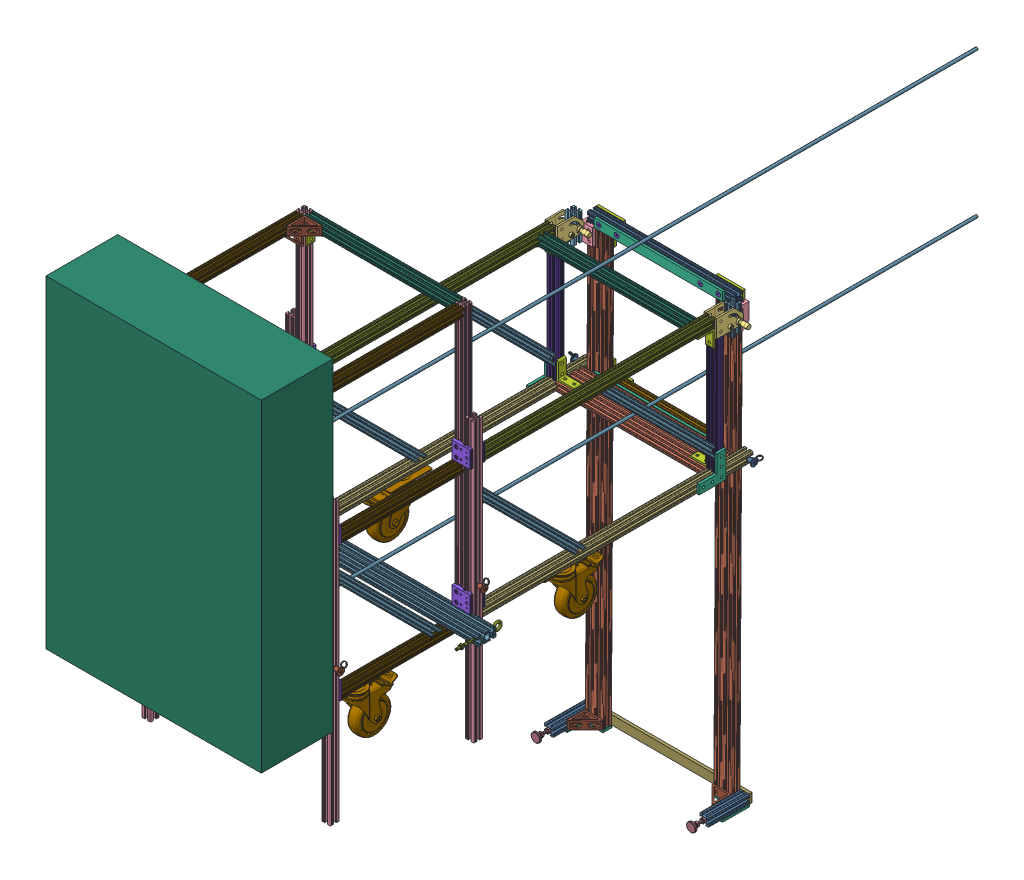
SolidWorks assembly _Tow System Assy V1.1, configuration Default. Lengths in mm.
Overall size (660.4 1762.18 2269.88).
108 component instances, 34 part files, 304 mates.
Components (placement in the parent):
- 8020 -1inch - 0 ft 4.5 in-1: 8020 -1inch - 0 ft 4.5 in [47065T122] at (5.4224 -1222.1152 -947.6338) x (-1 0 0) z (0 0.005452 0.999985) size (25.4 25.4 114.3)
- 8020 -1inch - 0 ft 4.5 in-2: 8020 -1inch - 0 ft 4.5 in [47065T122] at (445.4276 -1222.1152 -947.6338) x (-1 0 0) z (0 0.005452 0.999985) size (25.4 25.4 114.3)
- 47065T125_2inch - 4 ft-1: 47065T125_2inch - 4 ft [47065T125] at (43.5224 -625.4664 -995.3372) x (1 0 0) z (0 0.999985 -0.005452) size (50.8 25.4 1219.2)
- 47065T125_2inch - 4 ft-2: 47065T125_2inch - 4 ft [47065T125] at (407.3276 -625.4664 -995.3372) x (1 0 0) z (0 0.999985 -0.005452) size (50.8 25.4 1219.2)
- 3136N217_Heavy Duty 90 pivot-1: 3136N217_Heavy Duty 90 pivot [3136N217] at (0 -25.4 -927.1) x (-1 0 0) z (0 -1 0) size (70.02 76.2 50.8)
- 47065T953_1in Slider 90 degree-1: 47065T953_1in Slider 90 degree [47065T953] at (41.2872 -39.938 -998.377) x (0 -0.005452 -0.999985) z (0 0.999985 -0.005452) size (41.25 49.99 47.62)
- 47065T953_1in Slider 90 degree-3: 47065T953_1in Slider 90 degree [47065T953] at (409.5628 -39.938 -998.377) x (0 -0.005452 -0.999985) z (0 -0.999985 0.005452) size (41.25 49.99 47.62)
- 3136N217_Heavy Duty 90 pivot-2: 3136N217_Heavy Duty 90 pivot [3136N217] at (450.85 -25.4 -927.1) x (-1 0 0) z (0 -1 0) size (70.02 76.2 50.8)
- 8020 -1inch - 0 ft 3 in-1: 8020 -1inch - 0 ft 3 in [47065T122] at (0 -25.469 -965.1306) x (1 0 0) z (0 -0.999985 0.005452) size (25.4 25.4 76.2)
- 8020 -1inch - 0 ft 3 in-2: 8020 -1inch - 0 ft 3 in [47065T122] at (450.85 -25.469 -965.1306) x (1 0 0) z (0 -0.999985 0.005452) size (25.4 25.4 76.2)
- 1614T644_1in x 364mm Aluminium bar - 5_16 thick-1: 1614T644_1in x 364mm Aluminium bar - 5_16 thick [1614T644] at (225.5224 -380.9144 -980.9702) x (0 -0.999985 0.005452) z (-1 0 0) size (25.4 6 364)
- 1614T644_1in x 364mm Aluminium bar - 5_16 thick-2: 1614T644_1in x 364mm Aluminium bar - 5_16 thick [1614T644] at (225.5224 -3.09 -983.03) x (0 0.999985 -0.005452) z (1 0 0) size (25.4 6 364)
- T Bracket-21: T Bracket [Default] at (119.7224 -381.1039 -1015.7197) x (0 0.999985 -0.005452) z (0 0.005452 0.999985) size (76.2 76.2 6.35)
- T Bracket-22: T Bracket [Default] at (331.1276 -381.1039 -1015.7197) x (0 -0.999985 0.005452) z (0 0.005452 0.999985) size (76.2 76.2 6.35)
- 90585A358_SS Countersunk Screw 1_4-20 x 5-8 in-1: 90585A358_SS Countersunk Screw 1_4-20 x 5-8 in [90585A358] at (56.2224 -380.8981 -977.9703) x (-0.923728 0.383043 -0.002088) z (0 0.005452 0.999985) size (13.49 13.49 16.52)
- 90585A358_SS Countersunk Screw 1_4-20 x 5-8 in-3: 90585A358_SS Countersunk Screw 1_4-20 x 5-8 in [90585A358] at (394.8224 -380.8981 -977.9703) x (-0.923728 0.383043 -0.002088) z (0 0.005452 0.999985) size (13.49 13.49 16.52)
- 90585A358_SS Countersunk Screw 1_4-20 x 5-8 in-4: 90585A358_SS Countersunk Screw 1_4-20 x 5-8 in [90585A358] at (344.0224 -3.0737 -980.0301) x (-0.923728 0.383043 -0.002088) z (0 0.005452 0.999985) size (13.49 13.49 16.52)
- 90585A358_SS Countersunk Screw 1_4-20 x 5-8 in-5: 90585A358_SS Countersunk Screw 1_4-20 x 5-8 in [90585A358] at (344.0224 -380.8981 -977.9703) x (-0.923728 0.383043 -0.002088) z (0 0.005452 0.999985) size (13.49 13.49 16.52)
- 90585A358_SS Countersunk Screw 1_4-20 x 5-8 in-6: 90585A358_SS Countersunk Screw 1_4-20 x 5-8 in [90585A358] at (107.0224 -3.0737 -980.0301) x (-0.923728 0.383043 -0.002088) z (0 0.005452 0.999985) size (13.49 13.49 16.52)
- 90585A358_SS Countersunk Screw 1_4-20 x 5-8 in-7: 90585A358_SS Countersunk Screw 1_4-20 x 5-8 in [90585A358] at (56.2224 -3.0737 -980.0301) x (-0.923728 0.383043 -0.002088) z (0 0.005452 0.999985) size (13.49 13.49 16.52)
- 90585A358_SS Countersunk Screw 1_4-20 x 5-8 in-8: 90585A358_SS Countersunk Screw 1_4-20 x 5-8 in [90585A358] at (107.0224 -380.8981 -977.9703) x (-0.923728 0.383043 -0.002088) z (0 0.005452 0.999985) size (13.49 13.49 16.52)
- 90585A358_SS Countersunk Screw 1_4-20 x 5-8 in-9: 90585A358_SS Countersunk Screw 1_4-20 x 5-8 in [90585A358] at (394.8224 -3.0737 -980.0301) x (-0.923728 0.383043 -0.002088) z (0 0.005452 0.999985) size (13.49 13.49 16.52)
- 8020 -1inch - 1 ft 0.25-3: 8020 -1inch - 1 ft 0.25 [47065T122] at (224.4974 -381 -996.67) x (0 -0.005452 -0.999985) z (1 0 0) size (25.4 25.4 311.15)
- 8020 -1inch - 415mm-1: 8020 -1inch - 415mm [47065T122] at (225.6224 -3.1756 -998.7298) x (0 -0.005452 -0.999985) z (1 0 0) size (25.4 25.4 415)
- 47065T736_ Interior 90 guesset for 1 in-1: 47065T736_ Interior 90 guesset for 1 in [47065T736] at (18.1224 -1220.7008 -979.392) x (0 0.005452 0.999985) z (0 0.999985 -0.005452) size (50.8 50.8 22.23)
- 47065T736_ Interior 90 guesset for 1 in-2: 47065T736_ Interior 90 guesset for 1 in [47065T736] at (432.7276 -1220.7008 -979.392) x (0 0.005452 0.999985) z (0 -0.999985 0.005452) size (50.8 50.8 22.23)
- 1614T644_1in x 465mm Aluminium bar - 5_16 thick-1: 1614T644_1in x 465mm Aluminium bar - 5_16 thick [1614T644] at (225.2224 -1222.4484 -1008.7516) x (0 -0.999985 0.005452) z (-1 0 0) size (25.4 7.94 465)
- 6111K115_SS Leveling Foot-3: 6111K115_SS Leveling Foot [6111K115] at (5.4224 -1221.593 -851.856) x (0.003314 0.99998 -0.005452) z (-0.999995 0.003314 -0.000018) size (25.4 81.68 25.4)
- 6111K115_SS Leveling Foot-4: 6111K115_SS Leveling Foot [6111K115] at (445.4276 -1221.593 -851.856) x (0.316415 0.948607 -0.005172) z (-0.948621 0.316411 -0.001725) size (25.4 81.68 25.4)
- 8020 - 2inch - 2 ft 2 in-1: 8020 - 2inch - 2 ft 2 in [47065T213] at (225.425 -355.6 -165.1) x (0 0 1) z (-1 0 0) size (50.8 25.4 660.4)
- 8020 -1inch - 1 ft 4.75 in-9: 8020 -1inch - 1 ft 4.75 in [47065T122] at (225.425 -381 203.2) x (0 -1 0) z (1 0 0) size (25.4 25.4 425.45)
- 8020 -1inch - 2 ft 3 in-13: 8020 -1inch - 2 ft 3 in [47065T122] at (0 0 -558.8) x (-1 0 0) z (0 0 -1) size (25.4 25.4 685.8)
- 8020 -1inch - 2 ft 3 in-14: 8020 -1inch - 2 ft 3 in [47065T122] at (450.85 0 -558.8) x (-1 0 0) z (0 0 -1) size (25.4 25.4 685.8)
- 8020 -1inch - 1 ft 2 in-1: 8020 -1inch - 1 ft 2 in [47065T122] at (0 -190.5 -914.4) x (1 0 0) z (0 1 0) size (25.4 25.4 355.6)
- 8020 -1inch - 1 ft 3 in-2: 8020 -1inch - 1 ft 3 in [47065T122] at origin size (25.4 25.4 381)
- 8020 -1inch - 1 ft 3 in-3: 8020 -1inch - 1 ft 3 in [47065T122] at (0 -381 0) size (25.4 25.4 381)
- 8020 -1inch - 1 ft 2 in-2: 8020 -1inch - 1 ft 2 in [47065T122] at (450.85 -190.5 -914.4) x (1 0 0) z (0 1 0) size (25.4 25.4 355.6)
- 8020 -1inch - 1 ft 3 in-4: 8020 -1inch - 1 ft 3 in [47065T122] at (450.85 -381 0) size (25.4 25.4 381)
- 8020 -1inch - 1 ft 3 in-6: 8020 -1inch - 1 ft 3 in [47065T122] at (450.85 0 0) size (25.4 25.4 381)
- 8020 -1inch - 1 ft 4.75 in-18: 8020 -1inch - 1 ft 4.75 in [47065T122] at (225.425 0 -863.6) x (0 -1 0) z (1 0 0) size (25.4 25.4 425.45)
- 8020 - 2inch - 1 ft 4.75 in-9: 8020 - 2inch - 1 ft 4.75 in [47065T213] at (225.425 258.3 203.2) x (0 -1 0) z (1 0 0) size (50.8 25.4 425.45)
- 47065T512_8020 - 3inch - 1 ft 4.75 in-1: 47065T512_8020 - 3inch - 1 ft 4.75 in [47065T512] at (225.425 -381 -939.8) x (0 -1 0) z (-1 0 0) size (25.4 76.2 425.45)
- 8020 -1inch - 2 ft 8 inches-1: 8020 -1inch - 2 ft 8 inches [47065T122] at (0 -381 -612.635) size (25.4 25.4 793.47)
- 8020 -1inch - 2 ft 8 inches-2: 8020 -1inch - 2 ft 8 inches [47065T122] at (450.85 -381 -612.635) size (25.4 25.4 793.47)
- 8020 -1inch - 2 ft 7 inches-1: 8020 -1inch - 2 ft 7 inches [47065T122] at (0 0 -203.2) x (-1 0 0) z (0 1 0) size (25.4 25.4 787.4)
- 8020 -1inch - 2 ft 7 inches-2: 8020 -1inch - 2 ft 7 inches [47065T122] at (0 0 203.2) x (-1 0 0) z (0 1 0) size (25.4 25.4 787.4)
- 8020 -1inch - 2 ft 7 inches-3: 8020 -1inch - 2 ft 7 inches [47065T122] at (-29.21 -266.875 -203.3524) x (-1 0 0) z (0 1 0) size (25.4 25.4 787.4)
- 8020 -1inch - 1 ft 3 in-7: 8020 -1inch - 1 ft 3 in [47065T122] at (0 381 0) size (25.4 25.4 381)
- 8020 -1inch - 2 ft 7 inches-6: 8020 -1inch - 2 ft 7 inches [47065T122] at (450.85 0 -203.2) x (-1 0 0) z (0 1 0) size (25.4 25.4 787.4)
- 8020 -1inch - 1 ft 4.75 in-19: 8020 -1inch - 1 ft 4.75 in [47065T122] at (225.425 381 -203.2) x (0 -1 0) z (1 0 0) size (25.4 25.4 425.45)
- 8020 -1inch - 1 ft 4.75 in-20: 8020 -1inch - 1 ft 4.75 in [47065T122] at (225.425 381 203.2) x (0 -1 0) z (1 0 0) size (25.4 25.4 425.45)
- 47065T701_45 Brace - 18 in-12: 47065T701_45 Brace - 18 in [47065T701] at (450.85 -215.6355 -368.5645) x (1 0 0) z (0 0.707107 0.707107) size (25.4 25.56 457.2)
- 8020 -1inch - 2 ft 7 inches-8: 8020 -1inch - 2 ft 7 inches [47065T122] at (450.85 0 203.2) x (-1 0 0) z (0 1 0) size (25.4 25.4 787.4)
- 8020 -1inch - 1 ft 3 in-8: 8020 -1inch - 1 ft 3 in [47065T122] at (450.85 381 0) size (25.4 25.4 381)
- 8020 - 2inch - 1 ft 4.75 in-10: 8020 - 2inch - 1 ft 4.75 in [47065T213] at (225.425 -152.7 203.2) x (0 -1 0) z (1 0 0) size (50.8 25.4 425.45)
- 8020 - 2inch - 1 ft 4.75 in-11: 8020 - 2inch - 1 ft 4.75 in [47065T213] at (225.425 -228.9 203.2) x (0 -1 0) z (1 0 0) size (50.8 25.4 425.45)
- 8020 - 2inch - 1 ft 4.75 in-12: 8020 - 2inch - 1 ft 4.75 in [47065T213] at (225.425 182.1 203.2) x (0 -1 0) z (1 0 0) size (50.8 25.4 425.45)
- L Bracket-13: L Bracket [Default] at (68.9224 -1241.4072 -991.9793) x (0 -0.005452 -0.999985) z (0 0.999985 -0.005452) size (75.8 76.2 6.35)
- L Bracket-15: L Bracket [Default] at (381.9276 -1235.0573 -992.0139) x (0 -0.005452 -0.999985) z (0 -0.999985 0.005452) size (75.8 76.2 6.35)
- T Bracket-17: T Bracket [Default] at (19.05 -317.5 -203.2) x (0 0 -1) z (-1 0 0) size (76.2 76.2 6.35)
- 1 inch x 2 inch L bracket-10: 1 inch x 2 inch L bracket [47065T239] at (12.7 368.3 -204.7875) x (1 0 0) z (0 0 -1) size (50.8 50.8 22.23)
- L Bracket-17: L Bracket [Default] at (-12.7 -317.5 -914.4) x (0 0 -1) z (-1 0 0) size (75.8 76.2 6.35)
- L Bracket-18: L Bracket [Default] at (463.55 -381 -850.9) x (0 -1 0) z (1 0 0) size (75.8 76.2 6.35)
- 1 inch x 2 inch L bracket-39: 1 inch x 2 inch L bracket [47065T239] at (-1.5875 -12.7 -901.7) x (0 0 1) z (1 0 0) size (50.8 50.8 22.23)
- 1 inch x 2 inch L bracket-40: 1 inch x 2 inch L bracket [47065T239] at (452.4375 -12.7 -901.7) x (0 0 1) z (1 0 0) size (50.8 50.8 22.23)
- 1 inch x 2 inch L bracket-44: 1 inch x 2 inch L bracket [47065T239] at (12.7 -368.3 -915.9875) size (50.8 50.8 22.23)
- 1 inch x 2 inch L bracket-45: 1 inch x 2 inch L bracket [47065T239] at (438.15 -368.3 -915.9875) x (-1 0 0) z (0 0 -1) size (50.8 50.8 22.23)
- T Bracket-23: T Bracket [Default] at (394.6276 -66.7439 -1011.0834) x (-1 0 0) z (0 -0.005452 -0.999985) size (76.2 76.2 6.35)
- T Bracket-24: T Bracket [Default] at (56.2224 -66.7439 -1011.0834) x (-1 0 0) z (0 -0.005452 -0.999985) size (76.2 76.2 6.35)
- 47065T701_45 Brace - 18 in-10: 47065T701_45 Brace - 18 in [47065T701] at (0 165.3645 37.8355) x (1 0 0) z (0 0.707107 0.707107) size (25.4 25.56 457.2)
- 47065T701_45 Brace - 18 in-11: 47065T701_45 Brace - 18 in [47065T701] at (0 -215.6355 37.8355) x (1 0 0) z (0 0.707107 0.707107) size (25.4 25.56 457.2)
- 47065T736_ Interior 90 guesset for 1 in-3: 47065T736_ Interior 90 guesset for 1 in [47065T736] at (12.7 -379.4125 190.5) x (0 0 -1) z (0 -1 0) size (50.8 50.8 22.23)
- T Bracket-25: T Bracket [Default] at (12.7 0 139.7) x (0 1 0) z (1 0 0) size (76.2 76.2 6.35)
- L Bracket-19: L Bracket [Default] at (63.5 381 215.9) x (0 1 0) z (0 0 1) size (75.8 76.2 6.35)
- 47065T736_ Interior 90 guesset for 1 in-4: 47065T736_ Interior 90 guesset for 1 in [47065T736] at (-1.5875 368.3 -190.5) x (0 -1 0) z (-1 0 0) size (50.8 50.8 22.23)
- 47065T736_ Interior 90 guesset for 1 in-5: 47065T736_ Interior 90 guesset for 1 in [47065T736] at (12.7 382.5875 -190.5) x (1 0 0) z (0 -1 0) size (50.8 50.8 22.23)
- 47065T701_45 Brace - 18 in-1: 47065T701_45 Brace - 18 in [47065T701] at (0 -215.6355 -368.5645) x (1 0 0) z (0 0.707107 0.707107) size (25.4 25.56 457.2)
- 47065T701_45 Brace - 18 in-2: 47065T701_45 Brace - 18 in [47065T701] at (450.85 -215.6355 37.8355) x (1 0 0) z (0 0.707107 0.707107) size (25.4 25.56 457.2)
- 47065T701_45 Brace - 18 in-8: 47065T701_45 Brace - 18 in [47065T701] at (0 -165.3645 -749.0355) x (-1 0 0) z (0 0.707107 0.707107) size (25.4 25.56 457.2)
- 47065T701_45 Brace - 18 in-9: 47065T701_45 Brace - 18 in [47065T701] at (450.85 -165.3645 -749.0355) x (-1 0 0) z (0 0.707107 0.707107) size (25.4 25.56 457.2)
- 47065T778_1 in Slider-1: 47065T778_1 in Slider [47065T778] at (2.7154 35.2623 -202.0732) x (0 0 1) z (0 -1 0) size (41.25 52.61 48.02)
- 47065T778_1 in Slider-2: 47065T778_1 in Slider [47065T778] at (2.7154 -320.3377 -202.0732) x (0 0 1) z (0 -1 0) size (41.25 52.61 48.02)
- 8020 -1inch - 2 ft 7 inches-5: 8020 -1inch - 2 ft 7 inches [47065T122] at (-29.21 -266.875 203.3524) x (-1 0 0) z (0 1 0) size (25.4 25.4 787.4)
- 47065T778_1 in Slider-3: 47065T778_1 in Slider [47065T778] at (2.7154 -345.7377 204.3268) x (0 0 1) z (0 -1 0) size (41.25 52.61 48.02)
- 47065T778_1 in Slider-4: 47065T778_1 in Slider [47065T778] at (2.7154 35.2623 204.3268) x (0 0 1) z (0 -1 0) size (41.25 52.61 48.02)
- 8020 -1inch - 2 ft 7 inches-7: 8020 -1inch - 2 ft 7 inches [47065T122] at (480.06 -266.875 203.3524) x (-1 0 0) z (0 1 0) size (25.4 25.4 787.4)
- 47065T778_1 in Slider-5: 47065T778_1 in Slider [47065T778] at (448.1346 -320.3377 -204.3268) x (0 0 -1) z (0 -1 0) size (41.25 52.61 48.02)
- 47065T778_1 in Slider-6: 47065T778_1 in Slider [47065T778] at (448.1346 35.2623 -204.3268) x (0 0 -1) z (0 -1 0) size (41.25 52.61 48.02)
- 47065T778_1 in Slider-7: 47065T778_1 in Slider [47065T778] at (448.1346 -345.7377 202.0732) x (0 0 -1) z (0 -1 0) size (41.25 52.61 48.02)
- 47065T778_1 in Slider-8: 47065T778_1 in Slider [47065T778] at (448.1346 35.2623 202.0732) x (0 0 -1) z (0 -1 0) size (41.25 52.61 48.02)
- 8020 -1inch - 2 ft 7 inches-9: 8020 -1inch - 2 ft 7 inches [47065T122] at (480.06 -266.875 -203.0476) x (-1 0 0) z (0 1 0) size (25.4 25.4 787.4)
- 5537T435_ Caster Wheel 265lb Cap-1: 5537T435_ Caster Wheel 265lb Cap [5537T435] at (-1.2 -479.7 -479.1893) size (57 136 166.07)
- 5537T435_ Caster Wheel 265lb Cap-2: 5537T435_ Caster Wheel 265lb Cap [5537T435] at (-1.2 -479.7 80.5) size (57 136 166.07)
- 5537T435_ Caster Wheel 265lb Cap-3: 5537T435_ Caster Wheel 265lb Cap [5537T435] at (452.05 -479.7 -479.1893) x (-1 0 0) z (0 0 -1) size (57 136 166.07)
- 5537T435_ Caster Wheel 265lb Cap-4: 5537T435_ Caster Wheel 265lb Cap [5537T435] at (452.05 -479.7 105.1) x (-1 0 0) z (0 0 -1) size (57 136 166.07)
- 92851A140_SS HIGH-TENSION PUSH-BUTTON QUICK-RELEASE PIN - 4in usable length-1: 92851A140_SS HIGH-TENSION PUSH-BUTTON QUICK-RELEASE PIN - 4in usable length [92851A140] at (31.4642 -381 -996.67) x (-1 0 0) z (0 -0.482565 0.87586) size (134.21 33.71 20.64)
- 92851A140_SS HIGH-TENSION PUSH-BUTTON QUICK-RELEASE PIN - 4in usable length-2: 92851A140_SS HIGH-TENSION PUSH-BUTTON QUICK-RELEASE PIN - 4in usable length [92851A140] at (419.3858 -381 -996.67) x (1 0 0) z (0 -0.979653 -0.200697) size (134.21 33.71 20.64)
- 92851A125_SS HIGH-TENSION PUSH-BUTTON QUICK-RELEASE PIN - 2in length-1: 92851A125_SS HIGH-TENSION PUSH-BUTTON QUICK-RELEASE PIN - 2in length [92851A125] at (-23.1457 -279.4 -203.2) x (-1 0 0) z (0 0.952936 -0.303171) size (83.41 33.71 20.64)
- 92851A125_SS HIGH-TENSION PUSH-BUTTON QUICK-RELEASE PIN - 2in length-2: 92851A125_SS HIGH-TENSION PUSH-BUTTON QUICK-RELEASE PIN - 2in length [92851A125] at (-23.1457 -279.4 203.2) x (-1 0 0) z (0 -0.541594 -0.84064) size (83.41 33.71 20.64)
- 92851A125_SS HIGH-TENSION PUSH-BUTTON QUICK-RELEASE PIN - 2in length-3: 92851A125_SS HIGH-TENSION PUSH-BUTTON QUICK-RELEASE PIN - 2in length [92851A125] at (473.9957 -279.4 203.2) x (1 0 0) z (0 -0.585847 -0.810422) size (83.41 33.71 20.64)
- 92851A125_SS HIGH-TENSION PUSH-BUTTON QUICK-RELEASE PIN - 2in length-4: 92851A125_SS HIGH-TENSION PUSH-BUTTON QUICK-RELEASE PIN - 2in length [92851A125] at (473.9957 -279.4 -203.2) x (1 0 0) z (0 -0.36494 -0.931031) size (83.41 33.71 20.64)
- 1614T644_1in x 48mm Aluminium bar - 5_16 thick-1: 1614T644_1in x 48mm Aluminium bar - 5_16 thick [1614T644] at (0 16.6687 116.075) size (25.4 7.94 48)
- 47065T237_8020 2 in interior corner bracket-1: 47065T237_8020 2 in interior corner bracket [47065T237] at (12.7 20.6375 115.8875) x (0 1 0) z (0 0 1) size (25.4 25.4 47.62)
- Tether Placeholder-1: Tether Placeholder [Default] at (287.525 -284.9395 -1819.025) size (7.6 7.6 2000)
- Tether Placeholder-2: Tether Placeholder [Default] at (287.525 126.0605 -1819.025) x (0.198366 0.980128 0) z (0 0 1) size (7.6 7.6 2000)
- Electrical Enclosure Placeholder-1: Electrical Enclosure Placeholder [Default] at (-77.7 -393.7 247.65) x (1 0 0) z (0 -1 0) size (609.6 203.2 914.4)
- 3032T610_316 SS EYEBOLT W NUT 1-4_20 x 4 in-1: 3032T610_316 SS EYEBOLT W NUT 1-4_20 x 4 in [3032T61] at (542.925 -355.6 -206.375) x (0 -1 0) z (1 0 0) size (25.4 130.82 12.83)
- 3032T610_316 SS EYEBOLT W NUT 1-4_20 x 4 in-2: 3032T610_316 SS EYEBOLT W NUT 1-4_20 x 4 in [3032T61] at (-92.075 -355.6 -206.375) x (0 -1 0) z (1 0 0) size (25.4 130.82 12.83)
Mates (geometry in assembly coordinates):
- Concentric12: concentric anti-aligned: circle of L Bracket Spacer-3; circle of 1 inch x 2 inch L bracket-6
- Concentric13: concentric anti-aligned: circle of L Bracket Spacer-3; circle of 1 inch x 2 inch L bracket-6
- Coincident329: coincident anti-aligned: plane of L Bracket Spacer-3 through (558.333 1657.0643 1927.6829) normal (-0.646537 0.60797 -0.460828); plane of 1 inch x 2 inch L bracket-6 through (600.4865 1679.6629 1898.3561) normal (0.646537 -0.60797 0.460828)
- Concentric15: concentric anti-aligned: circle of L Bracket Spacer-4; circle of 1 inch x 2 inch L bracket-5
- Concentric16: concentric anti-aligned: circle of L Bracket Spacer-4; circle of 1 inch x 2 inch L bracket-5
- Coincident330: coincident anti-aligned: plane of L Bracket Spacer-4 through (764.4476 1681.6047 1670.8822) normal (-0.646537 0.60797 -0.460828); plane of 1 inch x 2 inch L bracket-5 through (765.1438 1682.8596 1671.5609) normal (0.646537 -0.60797 0.460828)
- Coincident668: coincident anti-aligned: plane of 8020 -1inch - 2 ft 3 in-13 through (12.7 9.5504 -901.7) normal (1 0 0); plane of 8020 -1inch - 1 ft 4.75 in-18 through (12.7 6.4164 -854.1902) normal (-1 0 0)
- Coincident669: coincident aligned: plane of 8020 -1inch - 2 ft 3 in-13 through (6.3331 12.7 -901.7) normal (0 1 0); plane of 8020 -1inch - 1 ft 4.75 in-18 through (438.15 12.7 -857.2669) normal (0 1 0)
- Coincident682: coincident aligned: plane of 8020 -1inch - 0 ft 4.5 in-1 through (-4.128 -1234.5034 -890.4154) normal (0 -0.999985 0.005452); plane of 47065T125_2inch - 4 ft-1 through (62.0475 -1235.1265 -1004.7137) normal (0 -0.999985 0.005452)
- Coincident683: coincident aligned: plane of 8020 -1inch - 0 ft 4.5 in-1 through (11.8388 -1213.017 -1004.8342) normal (0 -0.005452 -0.999985); plane of 47065T125_2inch - 4 ft-1 through (65.7728 -15.9447 -1011.3604) normal (0 -0.005452 -0.999985)
- Coincident685: coincident anti-aligned: plane of 8020 -1inch - 0 ft 4.5 in-1 through (18.1224 -1231.3539 -890.4326) normal (1 0 0); plane of 47065T125_2inch - 4 ft-1 through (18.1224 -15.8409 -992.3275) normal (-1 0 0)
- Coincident686: coincident anti-aligned: plane of L Bracket-13 through (68.9224 -1235.0573 -992.0139) normal (0 0.999985 -0.005452); plane of 47065T125_2inch - 4 ft-1 through (62.0475 -1235.1265 -1004.7137) normal (0 -0.999985 0.005452)
- Coincident687: coincident aligned: plane of L Bracket-13 through (18.1224 -1235.1265 -1004.7137) normal (0 -0.005452 -0.999985); plane of 47065T125_2inch - 4 ft-1 through (24.4893 -15.9447 -1011.3604) normal (0 -0.005452 -0.999985)
- Coincident688: coincident: plane of 8020 -1inch - 0 ft 4.5 in-1 through (-7.2776 -1228.1366 -890.4501) normal (-1 0 0); line of L Bracket-13 through (-7.2776 -1241.4765 -1004.6791) axis (0 0.005452 0.999985)
- Coincident696: coincident aligned: plane of 8020 -1inch - 0 ft 4.5 in-2 through (435.8772 -1234.5034 -890.4154) normal (0 -0.999985 0.005452); plane of 47065T125_2inch - 4 ft-2 through (425.8527 -1235.1265 -1004.7137) normal (0 -0.999985 0.005452)
- Coincident700: coincident aligned: plane of 8020 -1inch - 0 ft 4.5 in-2 through (451.844 -1213.017 -1004.8342) normal (0 -0.005452 -0.999985); plane of 47065T125_2inch - 4 ft-2 through (409.4612 -15.9447 -1011.3604) normal (0 -0.005452 -0.999985)
- Coincident701: coincident anti-aligned: plane of 8020 -1inch - 0 ft 4.5 in-2 through (432.7276 -1212.2533 -890.5367) normal (-1 0 0); plane of 47065T125_2inch - 4 ft-2 through (432.7276 -15.91 -1004.9937) normal (1 0 0)
- Coincident708: coincident anti-aligned: plane of 8020 -1inch - 0 ft 4.5 in-2 through (451.7607 -1234.5034 -890.4154) normal (0 -0.999985 0.005452); plane of L Bracket-15 through (381.9276 -1235.0573 -992.0139) normal (0 0.999985 -0.005452)
- Coincident709: coincident aligned: plane of 8020 -1inch - 0 ft 4.5 in-2 through (458.1276 -1231.3539 -890.4326) normal (1 0 0); plane of L Bracket-15 through (458.1276 -1241.4765 -1004.6791) normal (1 0 0)
- Coincident710: coincident aligned: plane of L Bracket-15 through (432.7276 -1241.4765 -1004.6791) normal (0 -0.005452 -0.999985); plane of 47065T125_2inch - 4 ft-2 through (429.578 -15.9447 -1011.3604) normal (0 -0.005452 -0.999985)
- Parallel16: parallel aligned: plane of 47065T125_2inch - 4 ft-1 through (24.4893 -15.9447 -1011.3604) normal (0 -0.005452 -0.999985); plane of 47065T125_2inch - 4 ft-2 through (388.2945 -15.9447 -1011.3604) normal (0 -0.005452 -0.999985)
- Coincident767: coincident aligned: plane of 3136N217_Heavy Duty 90 pivot-1 through (-17.4625 -38.1 -901.7) normal (0 0 1); plane of 8020 -1inch - 1 ft 2 in-1 through (-9.5504 -12.7 -901.7) normal (0 0 1)
- Coincident774: coincident aligned: plane of 8020 -1inch - 2 ft 3 in-13 through (-9.5504 12.7 -901.7) normal (0 1 0); plane of 3136N217_Heavy Duty 90 pivot-1 through (46.0901 12.7 -901.7) normal (0 1 0)
- Coincident784: coincident anti-aligned: plane of 47065T125_2inch - 4 ft-1 through (24.4893 -15.9447 -1011.3604) normal (0 -0.005452 -0.999985); plane of 47065T953_1in Slider 90 degree-1 through (41.2872 -16.3229 -1011.3583) normal (0 0.005452 0.999985)
- Coincident786: coincident anti-aligned: plane of 47065T125_2inch - 4 ft-1 through (18.1224 -15.9275 -1008.2108) normal (-1 0 0); plane of 47065T953_1in Slider 90 degree-1 through (18.1224 -16.2702 -1001.6811) normal (1 0 0)
- Distance13: distance = 4 mm aligned: plane of 47065T953_1in Slider 90 degree-1 through (-8.7 8.3249 -978.015) normal (-1 0 0); plane of 8020 -1inch - 0 ft 3 in-1 through (-12.7 -63.5164 -955.3726) normal (-1 0 0)
- Coincident818: coincident: plane of 8020 -1inch - 2 ft 3 in-14 through (457.1831 12.7 -901.7) normal (0 1 0); plane of 3136N217_Heavy Duty 90 pivot-2 through (497.7021 12.7 -901.7) normal (0 1 0)
- Coincident819: coincident: plane of 3136N217_Heavy Duty 90 pivot-2 through (469.0745 -38.1 -901.7) normal (0 0 1); plane of 8020 -1inch - 1 ft 2 in-2 through (457.1831 -12.7 -901.7) normal (0 0 1)
- Coincident821: coincident aligned: plane of 8020 -1inch - 2 ft 3 in-14 through (463.55 9.5504 -901.7) normal (1 0 0); plane of 8020 -1inch - 0 ft 3 in-2 through (463.55 -63.6205 -974.4731) normal (1 0 0)
- Coincident826: coincident anti-aligned: plane of 47065T125_2inch - 4 ft-2 through (429.578 -15.9447 -1011.3604) normal (0 -0.005452 -0.999985); plane of 47065T953_1in Slider 90 degree-3 through (423.0502 -63.6932 -1011.1001) normal (0 0.005452 0.999985)
- Coincident827: coincident anti-aligned: plane of 47065T125_2inch - 4 ft-2 through (432.7276 -15.91 -1004.9937) normal (1 0 0); plane of 47065T953_1in Slider 90 degree-3 through (432.7276 -63.6405 -1001.4228) normal (-1 0 0)
- Distance14: distance = 4 mm aligned: plane of 47065T953_1in Slider 90 degree-3 through (459.55 -87.9761 -977.49) normal (1 0 0); plane of 8020 -1inch - 0 ft 3 in-2 through (463.55 -63.534 -958.5899) normal (1 0 0)
- Coincident831: coincident aligned: plane of 47065T125_2inch - 4 ft-1 through (62.0475 -15.9447 -1011.3604) normal (0 0.999985 -0.005452); plane of 47065T125_2inch - 4 ft-2 through (425.8527 -15.9447 -1011.3604) normal (0 0.999985 -0.005452)
- Coincident862: coincident aligned: plane of 8020 -1inch - 1 ft 4.75 in-9 through (438.15 -368.3 193.6496) normal (0 1 0); plane of 8020 -1inch - 1 ft 3 in-3 through (-6.3331 -368.3 190.5) normal (0 1 0)
- Coincident869: coincident aligned: plane of 8020 -1inch - 1 ft 4.75 in-9 through (438.15 -368.3 209.5331) normal (0 1 0); plane of 8020 -1inch - 1 ft 3 in-4 through (460.4004 -368.3 190.5) normal (0 1 0)
- Coincident880: coincident anti-aligned: plane of 8020 -1inch - 1 ft 2 in-1 through (-9.5504 -12.7 -901.7) normal (0 0 1); plane of 47065T701_45 Brace - 18 in-8 through (12.7 -300.0684 -901.7) normal (0 0 -1)
- Coincident881: coincident anti-aligned: plane of 8020 -1inch - 2 ft 3 in-13 through (-6.3331 -12.7 -901.7) normal (0 -1 0); plane of 47065T701_45 Brace - 18 in-8 through (12.7 -12.7 -614.3316) normal (0 1 0)
- Coincident883: coincident anti-aligned: plane of 8020 -1inch - 1 ft 2 in-2 through (457.1831 -12.7 -901.7) normal (0 0 1); plane of 47065T701_45 Brace - 18 in-9 through (463.55 -300.0684 -901.7) normal (0 0 -1)
- Coincident884: coincident aligned: plane of 8020 -1inch - 1 ft 2 in-2 through (463.55 -12.7 -904.8496) normal (1 0 0); plane of 47065T701_45 Brace - 18 in-9 through (463.55 -10.473 -580.6378) normal (1 0 0)
- Coincident885: coincident anti-aligned: plane of 8020 -1inch - 2 ft 3 in-14 through (460.4004 -12.7 -901.7) normal (0 -1 0); plane of 47065T701_45 Brace - 18 in-9 through (463.55 -12.7 -614.3316) normal (0 1 0)
- Coincident886: coincident anti-aligned: plane of 8020 -1inch - 2 ft 3 in-13 through (9.5504 -12.7 -901.7) normal (0 -1 0); plane of 8020 -1inch - 1 ft 2 in-1 through (-6.4164 -12.7 -904.9902) normal (0 1 0)
- Coincident887: coincident anti-aligned: plane of 8020 -1inch - 2 ft 3 in-14 through (460.4004 -12.7 -901.7) normal (0 -1 0); plane of 8020 -1inch - 1 ft 2 in-2 through (444.4336 -12.7 -904.9902) normal (0 1 0)
- Coincident914: coincident aligned: plane of 8020 -1inch - 2 ft 3 in-13 through (-12.7 -9.5504 -901.7) normal (-1 0 0); plane of 1 inch x 2 inch L bracket-39 through (-12.7 -58.7248 -901.7) normal (-1 0 0)
- Coincident915: coincident anti-aligned: plane of 8020 -1inch - 1 ft 2 in-1 through (-9.5504 -12.7 -901.7) normal (0 0 1); plane of 1 inch x 2 inch L bracket-39 through (9.525 -12.7 -901.7) normal (0 0 -1)
- Coincident916: coincident anti-aligned: plane of 8020 -1inch - 2 ft 3 in-13 through (-6.3331 -12.7 -901.7) normal (0 -1 0); plane of 1 inch x 2 inch L bracket-39 through (9.525 -12.7 -850.9) normal (0 1 0)
- Coincident922: coincident aligned: plane of 8020 -1inch - 1 ft 2 in-2 through (457.1831 -12.7 -901.7) normal (0 0 1); plane of L Bracket-18 through (469.9 -317.9 -901.7) normal (0 0 1)
- Coincident923: coincident aligned: plane of 8020 -1inch - 2 ft 3 in-14 through (463.55 -6.3331 -901.7) normal (1 0 0); plane of 1 inch x 2 inch L bracket-40 through (463.55 -58.7248 -901.7) normal (1 0 0)
- Coincident924: coincident anti-aligned: plane of 8020 -1inch - 2 ft 3 in-14 through (460.4004 -12.7 -901.7) normal (0 -1 0); plane of 1 inch x 2 inch L bracket-40 through (463.55 -12.7 -850.9) normal (0 1 0)
- Coincident925: coincident anti-aligned: plane of 8020 -1inch - 1 ft 2 in-2 through (457.1831 -12.7 -901.7) normal (0 0 1); plane of 1 inch x 2 inch L bracket-40 through (463.55 -12.7 -901.7) normal (0 0 -1)
- Coincident934: coincident anti-aligned: plane of 47065T953_1in Slider 90 degree-1 through (7.9624 -16.0134 -977.8823) normal (0 0.005452 0.999985); plane of 8020 -1inch - 0 ft 3 in-1 through (-9.5504 -63.6377 -977.6227) normal (0 -0.005452 -0.999985)
- Coincident935: coincident aligned: plane of 47065T953_1in Slider 90 degree-1 through (41.2872 -63.6377 -977.6227) normal (0 -0.999985 0.005452); plane of 8020 -1inch - 0 ft 3 in-1 through (-6.4164 -63.6198 -974.3326) normal (0 -0.999985 0.005452)
- Coincident936: coincident aligned: line of 3136N217_Heavy Duty 90 pivot-1 through (-12.7 -12.7 -952.5) axis (1 0 0); line of 8020 -1inch - 0 ft 3 in-1 through (-9.5504 -12.7 -952.5) axis (1 0 0)
- Coincident937: coincident anti-aligned: plane of 47065T953_1in Slider 90 degree-3 through (442.8876 -63.6377 -977.6227) normal (0 0.005452 0.999985); plane of 8020 -1inch - 0 ft 3 in-2 through (457.1831 -63.6377 -977.6227) normal (0 -0.005452 -0.999985)
- Coincident938: coincident aligned: plane of 47065T953_1in Slider 90 degree-3 through (409.5628 -63.6377 -977.6227) normal (0 -0.999985 0.005452); plane of 8020 -1inch - 0 ft 3 in-2 through (444.4336 -63.6198 -974.3326) normal (0 -0.999985 0.005452)
- Coincident939: coincident: line of 3136N217_Heavy Duty 90 pivot-2 through (455.5744 -12.7 -952.5) axis (1 0 0); line of 8020 -1inch - 0 ft 3 in-2 through (457.1831 -12.7 -952.5) axis (1 0 0)
- Concentric28: concentric aligned: circle of 6111K115_SS Leveling Foot-3; circle of 8020 -1inch - 0 ft 4.5 in-1
- Coincident943: coincident anti-aligned: plane of 8020 -1inch - 0 ft 4.5 in-1 through (11.8388 -1212.3939 -890.5359) normal (0 0.005452 0.999985); plane of 6111K115_SS Leveling Foot-3 through (-0.9934 -1221.7823 -890.4847) normal (0 -0.005452 -0.999985)
- Concentric29: concentric aligned: circle of 6111K115_SS Leveling Foot-4; circle of 8020 -1inch - 0 ft 4.5 in-2
- Coincident944: coincident anti-aligned: plane of 8020 -1inch - 0 ft 4.5 in-2 through (451.844 -1212.3939 -890.5359) normal (0 0.005452 0.999985); plane of 6111K115_SS Leveling Foot-4 through (439.3414 -1219.7736 -890.4957) normal (0 -0.005452 -0.999985)
- Coincident955: coincident anti-aligned: plane of 47065T125_2inch - 4 ft-2 through (388.2945 -15.9447 -1011.3604) normal (0 -0.005452 -0.999985); plane of T Bracket-22 through (331.1276 -381.0692 -1009.3698) normal (0 0.005452 0.999985)
- Coincident957: coincident aligned: plane of 47065T125_2inch - 4 ft-2 through (381.9276 -15.9275 -1008.2108) normal (-1 0 0); plane of T Bracket-22 through (381.9276 -368.3694 -1009.439) normal (-1 0 0)
- Coincident960: coincident aligned: plane of 47065T125_2inch - 4 ft-1 through (68.9224 -15.91 -1004.9937) normal (1 0 0); plane of T Bracket-21 through (68.9224 -342.9698 -1009.5775) normal (1 0 0)
- Coincident971: coincident anti-aligned: plane of 8020 -1inch - 1 ft 2 in-1 through (12.7 -12.7 -920.7331) normal (1 0 0); plane of 1 inch x 2 inch L bracket-44 through (12.7 -368.3 -904.875) normal (-1 0 0)
- Coincident973: coincident aligned: plane of 8020 -1inch - 1 ft 2 in-1 through (9.5504 -12.7 -927.1) normal (0 0 -1); plane of 1 inch x 2 inch L bracket-44 through (12.7 -322.2752 -927.1) normal (0 0 -1)
- Coincident974: coincident anti-aligned: plane of 8020 -1inch - 1 ft 2 in-2 through (438.15 -12.7 -923.9504) normal (-1 0 0); plane of 1 inch x 2 inch L bracket-45 through (438.15 -368.3 -927.1) normal (1 0 0)
- Coincident975: coincident aligned: plane of 8020 -1inch - 1 ft 2 in-2 through (444.5169 -12.7 -927.1) normal (0 0 -1); plane of 1 inch x 2 inch L bracket-45 through (438.15 -322.2752 -927.1) normal (0 0 -1)
- Coincident1026: coincident aligned: plane of 47065T125_2inch - 4 ft-1 through (65.7728 -15.9447 -1011.3604) normal (0 -0.005452 -0.999985); plane of 8020 -1inch - 1 ft 0.25-3 through (380.0724 -390.6195 -1009.3177) normal (0 -0.005452 -0.999985)
- Coincident1027: coincident anti-aligned: plane of 47065T125_2inch - 4 ft-1 through (68.9224 -15.91 -1004.9937) normal (1 0 0); plane of 8020 -1inch - 1 ft 0.25-3 through (68.9224 -390.3747 -990.2024) normal (-1 0 0)
- Coincident1029: coincident aligned: plane of T Bracket-21 through (119.7224 -393.769 -1009.3006) normal (0 -0.999985 0.005452); plane of 8020 -1inch - 1 ft 0.25-3 through (380.0724 -393.7343 -1002.9338) normal (0 -0.999985 0.005452)
- Coincident1030: coincident anti-aligned: plane of 47065T125_2inch - 4 ft-1 through (65.7728 -15.9447 -1011.3604) normal (0 -0.005452 -0.999985); plane of T Bracket-21 through (119.7224 -381.0692 -1009.3698) normal (0 0.005452 0.999985)
- Coincident1031: coincident aligned: plane of T Bracket-22 through (381.9276 -393.769 -1009.3006) normal (0 -0.999985 0.005452); plane of 8020 -1inch - 1 ft 0.25-3 through (380.0724 -393.7343 -1002.9338) normal (0 -0.999985 0.005452)
- Distance42: distance = 25.4 mm aligned: plane of 1614T644_1in x 364mm Aluminium bar - 5_16 thick-1 through (43.5224 -380.9144 -980.9702) normal (-1 0 0); plane of 8020 -1inch - 1 ft 2.5-3 through (68.9224 -390.3747 -990.2024) normal (-1 0 0)
- Distance44: distance = 25.4 mm anti-aligned: plane of 1614T644_1in x 364mm Aluminium bar - 5_16 thick-2 through (43.5224 -3.09 -983.03) normal (-1 0 0); plane of 47065T125_2inch - 4 ft-1 through (68.9224 -15.8234 -989.1103) normal (1 0 0)
- Coincident1083: coincident anti-aligned: plane of 47065T125_2inch - 4 ft-1 through (62.0475 -15.9447 -1011.3604) normal (0 0.999985 -0.005452); plane of 8020 -1inch - 415mm-1 through (433.1224 -15.8234 -989.1103) normal (0 -0.999985 0.005452)
- Coincident1085: coincident aligned: plane of 47065T125_2inch - 4 ft-1 through (24.4893 -15.9447 -1011.3604) normal (0 -0.005452 -0.999985); plane of 8020 -1inch - 415mm-1 through (433.1224 3.0881 -1011.4641) normal (0 -0.005452 -0.999985)
- Distance45: distance = 352.43 mm anti-aligned: plane of 8020 -1inch - 1 ft 0.25-3 through (380.0724 -368.2657 -990.4062) normal (0 0.999985 -0.005452); plane of 8020 -1inch - 415mm-1 through (433.1224 -15.91 -1004.9936) normal (0 -0.999985 0.005452)
- Coincident1096: coincident anti-aligned: plane of 8020 -1inch - 415mm-1 through (433.1224 -12.7951 -1011.3776) normal (0 -0.005452 -0.999985); plane of T Bracket-24 through (56.2224 -66.7439 -1011.0834) normal (0 0.005452 0.999985)
- Coincident1099: coincident aligned: plane of 47065T125_2inch - 4 ft-1 through (68.9224 -15.91 -1004.9937) normal (1 0 0); plane of T Bracket-24 through (68.9224 -66.7785 -1017.4333) normal (1 0 0)
- Coincident1100: coincident anti-aligned: plane of 47065T125_2inch - 4 ft-2 through (388.2945 -15.9447 -1011.3604) normal (0 -0.005452 -0.999985); plane of T Bracket-23 through (394.6276 -66.7439 -1011.0834) normal (0 0.005452 0.999985)
- Coincident1102: coincident aligned: plane of 47065T125_2inch - 4 ft-2 through (381.9276 -15.9275 -1008.2108) normal (-1 0 0); plane of T Bracket-23 through (381.9276 -15.9793 -1017.7103) normal (-1 0 0)
- Coincident1107: coincident anti-aligned: plane of 8020 -1inch - 1 ft 2 in-1 through (12.7 -12.7 -920.7331) normal (1 0 0); plane of 47065T512_8020 - 3inch - 1 ft 4.75 in-1 through (12.7 -370.9416 -901.7) normal (-1 0 0)
- Coincident1108: coincident anti-aligned: plane of 8020 -1inch - 1 ft 2 in-1 through (-6.4164 -368.3 -904.9902) normal (0 -1 0); plane of 47065T512_8020 - 3inch - 1 ft 4.75 in-1 through (12.7 -368.3 -946.1246) normal (0 1 0)
- Coincident1109: coincident aligned: plane of 8020 -1inch - 2 ft 3 in-13 through (-12.7 -9.5504 -901.7) normal (-1 0 0); plane of 8020 -1inch - 1 ft 2 in-1 through (-12.7 -12.7 -923.9504) normal (-1 0 0)
- Coincident1110: coincident anti-aligned: plane of 8020 -1inch - 2 ft 3 in-13 through (6.4164 -9.4098 -901.7) normal (0 0 -1); plane of 8020 -1inch - 1 ft 2 in-1 through (-9.5504 -12.7 -901.7) normal (0 0 1)
- Coincident1111: coincident aligned: plane of 8020 -1inch - 1 ft 2 in-1 through (6.3331 -12.7 -901.7) normal (0 0 1); plane of 47065T512_8020 - 3inch - 1 ft 4.75 in-1 through (12.7 -390.5504 -901.7) normal (0 0 1)
- Coincident1114: coincident anti-aligned: plane of 8020 -1inch - 1 ft 2 in-1 through (-6.4164 -368.3 -904.9902) normal (0 -1 0); plane of 8020 -1inch - 2 ft 8 inches-1 through (-6.3331 -368.3 -215.9) normal (0 1 0)
- Tangent1: tangent: curve of 47065T701_45 Brace - 18 in-1; plane of 8020 -1inch - 2 ft 8 inches-1 through (-6.3331 -368.3 -215.9) normal (0 1 0)
- Coincident1116: coincident aligned: plane of 8020 -1inch - 1 ft 2 in-1 through (-12.7 -12.7 -908.0669) normal (-1 0 0); plane of 47065T701_45 Brace - 18 in-8 through (-12.7 3.0333 -594.1441) normal (-1 0 0)
- Coincident1120: coincident anti-aligned: plane of 8020 -1inch - 2 ft 3 in-14 through (457.2664 -9.4098 -901.7) normal (0 0 -1); plane of 8020 -1inch - 1 ft 2 in-2 through (457.1831 -12.7 -901.7) normal (0 0 1)
- Coincident1121: coincident anti-aligned: plane of 47065T125_2inch - 4 ft-1 through (62.5555 -15.8062 -985.9608) normal (0 0.005452 0.999985); plane of 47065T736_ Interior 90 guesset for 1 in-1 through (68.9224 -1209.5884 -979.4525) normal (0 -0.005452 -0.999985)
- Coincident1122: coincident aligned: plane of 8020 -1inch - 0 ft 4.5 in-1 through (14.9728 -1209.1038 -890.5539) normal (0 0.999985 -0.005452); plane of 47065T736_ Interior 90 guesset for 1 in-1 through (20.9196 -1209.3375 -933.4284) normal (0 0.999985 -0.005452)
- Coincident1123: coincident anti-aligned: plane of 8020 -1inch - 0 ft 4.5 in-1 through (18.1224 -1215.4706 -890.5191) normal (1 0 0); plane of 47065T736_ Interior 90 guesset for 1 in-1 through (18.1224 -1209.5884 -979.4525) normal (-1 0 0)
- Coincident1125: coincident anti-aligned: plane of 47065T125_2inch - 4 ft-2 through (426.3607 -15.8062 -985.9608) normal (0 0.005452 0.999985); plane of 47065T736_ Interior 90 guesset for 1 in-2 through (381.9276 -1231.8131 -979.3314) normal (0 -0.005452 -0.999985)
- Coincident1126: coincident anti-aligned: plane of 8020 -1inch - 0 ft 4.5 in-2 through (432.7276 -1212.2533 -890.5367) normal (-1 0 0); plane of 47065T736_ Interior 90 guesset for 1 in-2 through (432.7276 -1231.8131 -979.3314) normal (1 0 0)
- Coincident1127: coincident aligned: plane of 8020 -1inch - 0 ft 4.5 in-2 through (439.0945 -1209.1038 -890.5539) normal (0 0.999985 -0.005452); plane of 47065T736_ Interior 90 guesset for 1 in-2 through (429.9304 -1209.3375 -933.4284) normal (0 0.999985 -0.005452)
- Coincident1128: coincident anti-aligned: plane of 8020 -1inch - 0 ft 4.5 in-1 through (11.8388 -1213.017 -1004.8342) normal (0 -0.005452 -0.999985); plane of 1614T644_1in x 465mm Aluminium bar - 5_16 thick-1 through (-7.2776 -1235.1265 -1004.7137) normal (0 0.005452 0.999985)
- Coincident1129: coincident: plane of 8020 -1inch - 0 ft 4.5 in-1 through (-4.128 -1234.5034 -890.4154) normal (0 -0.999985 0.005452); line of 1614T644_1in x 465mm Aluminium bar - 5_16 thick-1 through (-7.2776 -1235.1698 -1012.6511) axis (1 0 0)
- Coincident1130: coincident aligned: plane of 8020 -1inch - 0 ft 4.5 in-1 through (-7.2776 -1228.1366 -890.4501) normal (-1 0 0); plane of 1614T644_1in x 465mm Aluminium bar - 5_16 thick-1 through (-7.2776 -1222.4484 -1008.7516) normal (-1 0 0)
- Coincident1131: coincident anti-aligned: circle of 8020 -1inch - 1 ft 2 in-2; plane of 8020 -1inch - 2 ft 8 inches-2 through (460.4004 -368.3 -215.9) normal (0 1 0)
- Coincident1132: coincident aligned: plane of 8020 -1inch - 1 ft 2 in-2 through (463.55 -12.7 -920.7331) normal (1 0 0); plane of 8020 -1inch - 2 ft 8 inches-2 through (463.55 -374.6669 -215.9) normal (1 0 0)
- Coincident1133: coincident aligned: circle of 8020 -1inch - 2 ft 8 inches-1; plane of 8020 -1inch - 2 ft 8 inches-2 through (444.4336 -390.4098 -1009.37) normal (0 0 -1)
- Coincident1134: coincident aligned: plane of 8020 -1inch - 2 ft 3 in-14 through (463.55 -6.3331 -901.7) normal (1 0 0); plane of 8020 -1inch - 1 ft 2 in-2 through (463.55 -12.7 -904.8496) normal (1 0 0)
- Concentric41: concentric aligned: cylinder of 8020 -1inch - 2 ft 8 inches-1 through (-12.7 -381 -996.67) axis (1 0 0) radius 3.5; cylinder of 92851A140_SS HIGH-TENSION PUSH-BUTTON QUICK-RELEASE PIN - 4in usable length-1 through (-33.3375 -381 -996.67) axis (1 0 0) radius 3.1559
- Coincident1137: coincident anti-aligned: plane of 8020 -1inch - 2 ft 8 inches-1 through (-12.7 -371.4496 -215.9) normal (-1 0 0); plane of 92851A140_SS HIGH-TENSION PUSH-BUTTON QUICK-RELEASE PIN - 4in usable length-1 through (-12.7 -385.242 -999.0072) normal (1 0 0)
- Concentric42: concentric anti-aligned: cylinder of 8020 -1inch - 2 ft 8 inches-2 through (438.15 -381 -996.67) axis (1 0 0) radius 3.5; cylinder of 92851A140_SS HIGH-TENSION PUSH-BUTTON QUICK-RELEASE PIN - 4in usable length-2 through (484.1875 -381 -996.67) axis (-1 0 0) radius 3.1559
- Coincident1138: coincident anti-aligned: plane of 8020 -1inch - 2 ft 8 inches-2 through (463.55 -374.6669 -215.9) normal (1 0 0); plane of 92851A140_SS HIGH-TENSION PUSH-BUTTON QUICK-RELEASE PIN - 4in usable length-2 through (463.55 -381.972 -991.9254) normal (-1 0 0)
- Coincident1144: coincident aligned: plane of 8020 -1inch - 2 ft 3 in-14 through (441.2996 12.7 -901.7) normal (0 1 0); plane of 8020 -1inch - 1 ft 4.75 in-18 through (438.15 12.7 -873.1504) normal (0 1 0)
- Coincident1145: coincident anti-aligned: plane of 8020 -1inch - 1 ft 3 in-2 through (-6.3331 12.7 190.5) normal (0 1 0); plane of 47065T701_45 Brace - 18 in-10 through (-12.7 12.7 -96.8684) normal (0 -1 0)
- Coincident1146: coincident aligned: plane of 8020 -1inch - 1 ft 3 in-2 through (-12.7 9.5504 190.5) normal (-1 0 0); plane of 47065T701_45 Brace - 18 in-10 through (-12.7 333.7622 192.727) normal (-1 0 0)
